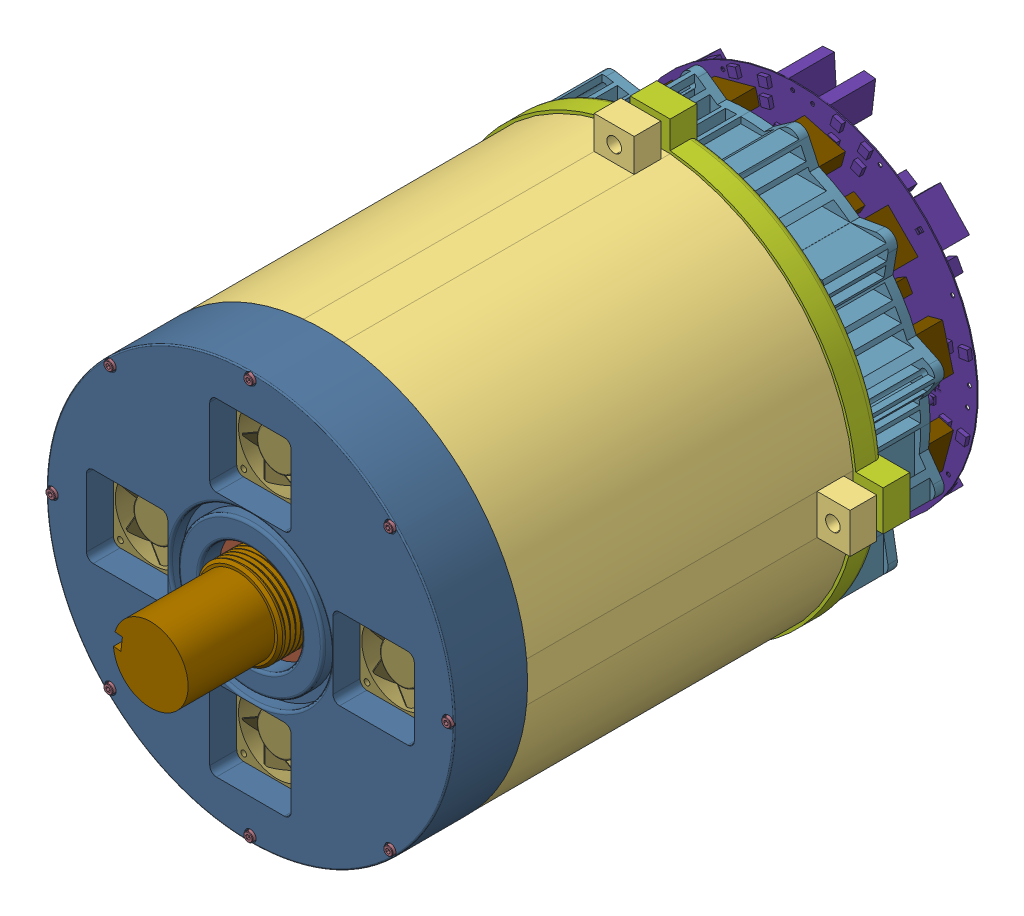
SolidWorks assembly motor assembly, configuration Varsayılan. Lengths in mm.
Overall size (354 354 520.07).
111 component instances, 18 part files, 52 mates.
Components (placement in the parent):
- stator-1: stator [Varsayılan] at (-45.285 13.1183 202.5) size (270 270 135)
- coil-1: coil [Varsayılan] at (-45.285 -93.8817 270) size (21.5 30 205)
- coil-2: coil [Varsayılan] at (-17.5914 -90.2358 270) x (0.965926 0.258819 0) z (0 0 1) size (21.5 30 205)
- coil-3: coil [Varsayılan] at (8.215 -79.5464 270) x (0.866025 0.5 0) z (0 0 1) size (21.5 30 205)
- coil-4: coil [Varsayılan] at (30.3754 -62.5422 270) x (0.707107 0.707107 0) z (0 0 1) size (21.5 30 205)
- coil-5: coil [Varsayılan] at (47.3797 -40.3817 270) x (0.5 0.866025 0) z (0 0 1) size (21.5 30 205)
- coil-6: coil [Varsayılan] at (58.0691 -14.5754 270) x (0.258819 0.965926 0) z (0 0 1) size (21.5 30 205)
- coil-7: coil [Varsayılan] at (61.715 13.1183 270) x (0 1 0) z (0 0 1) size (21.5 30 205)
- coil-8: coil [Varsayılan] at (58.0691 40.8119 270) x (-0.258819 0.965926 0) z (0 0 1) size (21.5 30 205)
- coil-9: coil [Varsayılan] at (47.3797 66.6183 270) x (-0.5 0.866025 0) z (0 0 1) size (21.5 30 205)
- coil-10: coil [Varsayılan] at (30.3754 88.7787 270) x (-0.707107 0.707107 0) z (0 0 1) size (21.5 30 205)
- coil-11: coil [Varsayılan] at (8.215 105.783 270) x (-0.866025 0.5 0) z (0 0 1) size (21.5 30 205)
- coil-12: coil [Varsayılan] at (-17.5914 116.4723 270) x (-0.965926 0.258819 0) z (0 0 1) size (21.5 30 205)
- coil-13: coil [Varsayılan] at (-45.285 120.1183 270) x (-1 0 0) z (0 0 1) size (21.5 30 205)
- coil-14: coil [Varsayılan] at (-72.9786 116.4723 270) x (-0.965926 -0.258819 0) z (0 0 1) size (21.5 30 205)
- coil-15: coil [Varsayılan] at (-98.785 105.783 270) x (-0.866025 -0.5 0) z (0 0 1) size (21.5 30 205)
- coil-16: coil [Varsayılan] at (-120.9454 88.7787 270) x (-0.707107 -0.707107 0) z (0 0 1) size (21.5 30 205)
- coil-17: coil [Varsayılan] at (-137.9497 66.6183 270) x (-0.5 -0.866025 0) z (0 0 1) size (21.5 30 205)
- coil-18: coil [Varsayılan] at (-148.6391 40.8119 270) x (-0.258819 -0.965926 0) z (0 0 1) size (21.5 30 205)
- coil-19: coil [Varsayılan] at (-152.285 13.1183 270) x (0 -1 0) z (0 0 1) size (21.5 30 205)
- coil-20: coil [Varsayılan] at (-148.6391 -14.5754 270) x (0.258819 -0.965926 0) z (0 0 1) size (21.5 30 205)
- coil-21: coil [Varsayılan] at (-137.9497 -40.3817 270) x (0.5 -0.866025 0) z (0 0 1) size (21.5 30 205)
- coil-22: coil [Varsayılan] at (-120.9454 -62.5422 270) x (0.707107 -0.707107 0) z (0 0 1) size (21.5 30 205)
- coil-23: coil [Varsayılan] at (-98.785 -79.5464 270) x (0.866025 -0.5 0) z (0 0 1) size (21.5 30 205)
- coil-24: coil [Varsayılan] at (-72.9786 -90.2358 270) x (0.965926 -0.258819 0) z (0 0 1) size (21.5 30 205)
- case-1: case [Varsayılan] at (-45.285 13.1183 390) x (-1 0 0) z (0 -1 0) size (354 245 354)
- rotor assembly-1: rotor assembly [Varsayılan] at (-60.6102 4.0993 71.3059) x (0.997912 -0.064595 0) z (0 0 1) size (229.36 229.36 135)
  - rotor core 1-1: rotor core 1 [Varsayılan] at (14.7106 9.9901 131.1941) size (164.94 164.94 67.5)
  - rotor core 2-1: rotor core 2 [Varsayılan] at (14.7106 9.9901 266.1941) x (0.824126 0.566406 0) z (0 0 -1) size (164.94 164.94 67.5)
  - magnet_67.5-1: magnet_67.5 [Varsayılan] at (14.7106 9.9901 198.6941) x (0.999657 -0.026177 0) z (0 0 1) size (19.71 16.61 67.5)
  - magnet_67.5-2: magnet_67.5 [Varsayılan] at (14.7106 9.9901 198.6941) x (0.95882 0.284015 0) z (0 0 1) size (19.71 16.61 67.5)
  - magnet_67.5-3: magnet_67.5 [Varsayılan] at (14.7106 9.9901 198.6941) x (0.824126 0.566406 0) z (0 0 1) size (19.71 16.61 67.5)
  - magnet_67.5-4: magnet_67.5 [Varsayılan] at (14.7106 9.9901 198.6941) x (0.608761 0.793353 0) z (0 0 1) size (19.71 16.61 67.5)
  - magnet_67.5-5: magnet_67.5 [Varsayılan] at (14.7106 9.9901 198.6941) x (0.333807 0.942641 0) z (0 0 1) size (19.71 16.61 67.5)
  - magnet_67.5-6: magnet_67.5 [Varsayılan] at (14.7106 9.9901 198.6941) x (0.026177 0.999657 0) z (0 0 1) size (19.71 16.61 67.5)
  - magnet_67.5-7: magnet_67.5 [Varsayılan] at (14.7106 9.9901 198.6941) x (-0.284015 0.95882 0) z (0 0 1) size (19.71 16.61 67.5)
  - magnet_67.5-8: magnet_67.5 [Varsayılan] at (14.7106 9.9901 198.6941) x (-0.566406 0.824126 0) z (0 0 1) size (19.71 16.61 67.5)
  - magnet_67.5-9: magnet_67.5 [Varsayılan] at (14.7106 9.9901 198.6941) x (-0.793353 0.608761 0) z (0 0 1) size (19.71 16.61 67.5)
  - magnet_67.5-10: magnet_67.5 [Varsayılan] at (14.7106 9.9901 198.6941) x (-0.942641 0.333807 0) z (0 0 1) size (19.71 16.61 67.5)
  - magnet_67.5-11: magnet_67.5 [Varsayılan] at (14.7106 9.9901 198.6941) x (-0.999657 0.026177 0) z (0 0 1) size (19.71 16.61 67.5)
  - magnet_67.5-12: magnet_67.5 [Varsayılan] at (14.7106 9.9901 198.6941) x (-0.95882 -0.284015 0) z (0 0 1) size (19.71 16.61 67.5)
  - magnet_67.5-13: magnet_67.5 [Varsayılan] at (14.7106 9.9901 198.6941) x (-0.824126 -0.566406 0) z (0 0 1) size (19.71 16.61 67.5)
  - magnet_67.5-14: magnet_67.5 [Varsayılan] at (14.7106 9.9901 198.6941) x (-0.608761 -0.793353 0) z (0 0 1) size (19.71 16.61 67.5)
  - magnet_67.5-15: magnet_67.5 [Varsayılan] at (14.7106 9.9901 198.6941) x (-0.333807 -0.942641 0) z (0 0 1) size (19.71 16.61 67.5)
  - magnet_67.5-16: magnet_67.5 [Varsayılan] at (14.7106 9.9901 198.6941) x (-0.026177 -0.999657 0) z (0 0 1) size (19.71 16.61 67.5)
  - magnet_67.5-17: magnet_67.5 [Varsayılan] at (14.7106 9.9901 198.6941) x (0.284015 -0.95882 0) z (0 0 1) size (19.71 16.61 67.5)
  - magnet_67.5-18: magnet_67.5 [Varsayılan] at (14.7106 9.9901 198.6941) x (0.566406 -0.824126 0) z (0 0 1) size (19.71 16.61 67.5)
  - magnet_67.5-19: magnet_67.5 [Varsayılan] at (14.7106 9.9901 198.6941) x (0.793353 -0.608761 0) z (0 0 1) size (19.71 16.61 67.5)
  - magnet_67.5-20: magnet_67.5 [Varsayılan] at (14.7106 9.9901 198.6941) x (0.942641 -0.333807 0) z (0 0 1) size (19.71 16.61 67.5)
  - magnet_67.5-21: magnet_67.5 [Varsayılan] at (14.7106 9.9901 131.1941) size (19.71 16.61 67.5)
  - magnet_67.5-22: magnet_67.5 [Varsayılan] at (14.7106 9.9901 131.1941) x (0.951057 -0.309017 0) z (0 0 1) size (19.71 16.61 67.5)
  - magnet_67.5-23: magnet_67.5 [Varsayılan] at (14.7106 9.9901 131.1941) x (0.809017 -0.587785 0) z (0 0 1) size (19.71 16.61 67.5)
  - magnet_67.5-24: magnet_67.5 [Varsayılan] at (14.7106 9.9901 131.1941) x (0.587785 -0.809017 0) z (0 0 1) size (19.71 16.61 67.5)
  - magnet_67.5-25: magnet_67.5 [Varsayılan] at (14.7106 9.9901 131.1941) x (0.309017 -0.951057 0) z (0 0 1) size (19.71 16.61 67.5)
  - magnet_67.5-26: magnet_67.5 [Varsayılan] at (14.7106 9.9901 131.1941) x (0 -1 0) z (0 0 1) size (19.71 16.61 67.5)
  - magnet_67.5-27: magnet_67.5 [Varsayılan] at (14.7106 9.9901 131.1941) x (-0.309017 -0.951057 0) z (0 0 1) size (19.71 16.61 67.5)
  - magnet_67.5-28: magnet_67.5 [Varsayılan] at (14.7106 9.9901 131.1941) x (-0.587785 -0.809017 0) z (0 0 1) size (19.71 16.61 67.5)
  - magnet_67.5-29: magnet_67.5 [Varsayılan] at (14.7106 9.9901 131.1941) x (-0.809017 -0.587785 0) z (0 0 1) size (19.71 16.61 67.5)
  - magnet_67.5-30: magnet_67.5 [Varsayılan] at (14.7106 9.9901 131.1941) x (-0.951057 -0.309017 0) z (0 0 1) size (19.71 16.61 67.5)
  - magnet_67.5-31: magnet_67.5 [Varsayılan] at (14.7106 9.9901 131.1941) x (-1 0 0) z (0 0 1) size (19.71 16.61 67.5)
  - magnet_67.5-32: magnet_67.5 [Varsayılan] at (14.7106 9.9901 131.1941) x (-0.951057 0.309017 0) z (0 0 1) size (19.71 16.61 67.5)
  - magnet_67.5-33: magnet_67.5 [Varsayılan] at (14.7106 9.9901 131.1941) x (-0.809017 0.587785 0) z (0 0 1) size (19.71 16.61 67.5)
  - magnet_67.5-34: magnet_67.5 [Varsayılan] at (14.7106 9.9901 131.1941) x (-0.587785 0.809017 0) z (0 0 1) size (19.71 16.61 67.5)
  - magnet_67.5-35: magnet_67.5 [Varsayılan] at (14.7106 9.9901 131.1941) x (-0.309017 0.951057 0) z (0 0 1) size (19.71 16.61 67.5)
  - magnet_67.5-36: magnet_67.5 [Varsayılan] at (14.7106 9.9901 131.1941) x (0 1 0) z (0 0 1) size (19.71 16.61 67.5)
  - magnet_67.5-37: magnet_67.5 [Varsayılan] at (14.7106 9.9901 131.1941) x (0.309017 0.951057 0) z (0 0 1) size (19.71 16.61 67.5)
  - magnet_67.5-38: magnet_67.5 [Varsayılan] at (14.7106 9.9901 131.1941) x (0.587785 0.809017 0) z (0 0 1) size (19.71 16.61 67.5)
  - magnet_67.5-39: magnet_67.5 [Varsayılan] at (14.7106 9.9901 131.1941) x (0.809017 0.587785 0) z (0 0 1) size (19.71 16.61 67.5)
  - magnet_67.5-40: magnet_67.5 [Varsayılan] at (14.7106 9.9901 131.1941) x (0.951057 0.309017 0) z (0 0 1) size (19.71 16.61 67.5)
- arka kapak zgr-1: arka kapak zgr [Default] at (-45.285 13.1183 160) x (0 0 -1) z (1 0 0) size (35.23 349.6 349.6)
- 6205 rulman-1: 6205 rulman [Varsayılan] at (-45.285 13.1183 135) x (0.999542 -0.030267 0) z (0 0 1) size (62 62 16)
- mıl-1: mıl [Default] at (-45.285 13.1183 499.75) x (0 0 1) z (-0.111143 -0.993804 0) size (443 80 80)
- on kapak-1: on kapak [Default] at (-45.285 13.1183 380) size (306 306 65)
- 6212 rulman-1: 6212 rulman [Default] at (-45.285 13.1183 408) size (110 110 22)
- 6212 rulman-2: 6212 rulman [Default] at (-45.285 13.1183 386) x (0.99317 -0.116678 0) z (0 0 1) size (110 110 22)
- Fan-60x60-1: Fan-60x60 [25mm] at (-45.285 105.6183 406.0237) size (71.21 64.96 25)
- Fan-60x60-2: Fan-60x60 [25mm] at (-137.785 13.1183 406.0237) x (0 1 0) z (0 0 1) size (71.21 64.96 25)
- Fan-60x60-3: Fan-60x60 [25mm] at (-45.285 -79.3817 406.0237) x (-1 0 0) z (0 0 1) size (71.21 64.96 25)
- Fan-60x60-4: Fan-60x60 [25mm] at (47.215 13.1183 406.0237) x (0 -1 0) z (0 0 1) size (71.21 64.96 25)
- Fan-60x60-5: Fan-60x60 [25mm] at (-101.8535 69.6868 131.0283) x (0 -1 0) z (0 0 1) size (71.21 64.96 25)
- socket head cap screw_am-1: socket head cap screw_am [B18.3.1M - 4 x 0.7 x 30 Hex SHCS -- 20CHX] at (63.0994 -49.154 42.8) x (0 0 1) z (0.759805 0.650151 0) size (34 7 7)
- socket head cap screw_am-3: socket head cap screw_am [B18.3.1M - 4 x 0.7 x 30 Hex SHCS -- 20CHX] at (75.3874 45.7245 42.8) x (0 0 1) z (0.077537 0.99699 0) size (34 7 7) (hidden)
- socket head cap screw_am-4: socket head cap screw_am [B18.3.1M - 4 x 0.7 x 30 Hex SHCS -- 20CHX] at (16.9872 121.5026 42.8) x (0 0 1) z (-0.650151 0.759805 0) size (34 7 7) (hidden)
- socket head cap screw_am-5: socket head cap screw_am [B18.3.1M - 4 x 0.7 x 30 Hex SHCS -- 20CHX] at (-77.8912 133.7907 42.8) x (0 0 1) z (-0.99699 0.077537 0) size (34 7 7) (hidden)
- socket head cap screw_am-6: socket head cap screw_am [B18.3.1M - 4 x 0.7 x 30 Hex SHCS -- 20CHX] at (-153.6694 75.3905 42.8) x (0 0 1) z (-0.759805 -0.650151 0) size (34 7 7) (hidden)
- socket head cap screw_am-7: socket head cap screw_am [B18.3.1M - 4 x 0.7 x 30 Hex SHCS -- 20CHX] at (-165.9574 -19.4879 42.8) x (0 0 1) z (-0.077537 -0.99699 0) size (34 7 7) (hidden)
- socket head cap screw_am-8: socket head cap screw_am [B18.3.1M - 4 x 0.7 x 30 Hex SHCS -- 20CHX] at (-107.5572 -95.2661 42.8) x (0 0 1) z (0.650151 -0.759805 0) size (34 7 7) (hidden)
- socket head cap screw_am-9: socket head cap screw_am [B18.3.1M - 4 x 0.7 x 30 Hex SHCS -- 20CHX] at (-12.6788 -107.5542 42.8) x (0 0 1) z (0.99699 -0.077537 0) size (34 7 7) (hidden)
- Fan-60x60-12: Fan-60x60 [25mm] at (-101.8535 -43.4503 131.0283) size (71.21 64.96 25)
- Fan-60x60-13: Fan-60x60 [25mm] at (11.2835 -43.4503 131.0283) x (0 1 0) z (0 0 1) size (71.21 64.96 25)
- Fan-60x60-14: Fan-60x60 [25mm] at (11.2835 69.6868 131.0283) x (-1 0 0) z (0 0 1) size (71.21 64.96 25)
- HeatSinkOneModule_mst-2: HeatSinkOneModule_mst [Varsayılan] at (-45.285 13.1183 70) x (1 0 0) z (0 -1 0) size (145.64 55 145.64)
- HeatSinkOneModule_mst-3: HeatSinkOneModule_mst [Varsayılan] at (-45.285 13.1183 70) x (0 1 0) z (1 0 0) size (145.64 55 145.64)
- HeatSinkOneModule_mst-4: HeatSinkOneModule_mst [Varsayılan] at (-45.285 13.1183 70) x (-1 0 0) z (0 1 0) size (145.64 55 145.64)
- HeatSinkOneModule_mst-5: HeatSinkOneModule_mst [Varsayılan] at (-45.285 13.1183 70) x (0 -1 0) z (-1 0 0) size (145.64 55 145.64)
- encoder_assem-1: encoder_assem [Varsayılan] at (-49.9209 11.8321 164) x (-0.034519 0.999404 0) z (0 0 -1) size (52.69 74.69 46.7)
  - encoder_body-1: encoder_body [Varsayılan] at (1.1254 4.6776 50) size (50 50 44.7)
  - encoder_bracket-1: encoder_bracket [Varsayılan] at (1.1254 4.6776 49.9) x (0 0 -1) z (-0.999404 -0.034519 0) size (11 73 50.2)
- ControlBoard-1: ControlBoard [Varsayılan] at (-45.2858 13.1179 33.7804) x (-0.027373 -0.999625 0) z (0 0 -1) size (270 270 45.4)
- GD_Layout-1: GD_Layout [Varsayılan] at (-45.2843 13.119 68.5789) x (0 1 0) z (0 0 -1) size (133 133 24.37)
- GD_Layout-2: GD_Layout [Varsayılan] at (-45.285 13.1183 68.5789) x (1 0 0) z (0 0 -1) size (133 133 24.37)
- GD_Layout-3: GD_Layout [Varsayılan] at (-45.285 13.1183 68.5789) x (0 -1 0) z (0 0 -1) size (133 133 24.37)
- GD_Layout-4: GD_Layout [Varsayılan] at (-45.2857 13.119 68.5789) x (-1 0 0) z (0 0 -1) size (133 133 24.37)
- socket head cap screw_am-10: socket head cap screw_am [B18.3.1M - 4 x 0.7 x 80 Hex SHCS -- 20NHX] at (-45.285 161.5955 446.8) x (0 0 -1) z (0.019286 0.999814 0) size (84 7 7)
- socket head cap screw_am-11: socket head cap screw_am [B18.3.1M - 4 x 0.7 x 80 Hex SHCS -- 20NHX] at (-150.2742 118.1075 446.8) x (0 0 -1) z (-0.693338 0.720612 0) size (84 7 7)
- socket head cap screw_am-12: socket head cap screw_am [B18.3.1M - 4 x 0.7 x 80 Hex SHCS -- 20NHX] at (-193.7622 13.1183 446.8) x (0 0 -1) z (-0.999814 0.019286 0) size (84 7 7)
- socket head cap screw_am-13: socket head cap screw_am [B18.3.1M - 4 x 0.7 x 80 Hex SHCS -- 20NHX] at (-150.2742 -91.8709 446.8) x (0 0 -1) z (-0.720612 -0.693338 0) size (84 7 7)
- socket head cap screw_am-14: socket head cap screw_am [B18.3.1M - 4 x 0.7 x 80 Hex SHCS -- 20NHX] at (-45.285 -135.3589 446.8) x (0 0 -1) z (-0.019286 -0.999814 0) size (84 7 7)
- socket head cap screw_am-15: socket head cap screw_am [B18.3.1M - 4 x 0.7 x 80 Hex SHCS -- 20NHX] at (59.7042 -91.8709 446.8) x (0 0 -1) z (0.693338 -0.720612 0) size (84 7 7)
- socket head cap screw_am-16: socket head cap screw_am [B18.3.1M - 4 x 0.7 x 80 Hex SHCS -- 20NHX] at (103.1922 13.1183 446.8) x (0 0 -1) z (0.999814 -0.019286 0) size (84 7 7)
- socket head cap screw_am-17: socket head cap screw_am [B18.3.1M - 4 x 0.7 x 80 Hex SHCS -- 20NHX] at (59.7042 118.1075 446.8) x (0 0 -1) z (0.720612 0.693338 0) size (84 7 7)
Mates (geometry in assembly coordinates):
- Width1: width: plane of coil-1 through (-38.535 -78.8817 270) normal (-1 0 0); plane of coil-1 through (-52.035 -78.8817 361.8) normal (1 0 0); plane of stator-1 through (-39.0069 -108.9108 337.5) normal (1 0 0); plane of stator-1 through (-51.5631 -76.6625 337.5) normal (-1 0 0)
- Width2: width: plane of stator-1 through (-45.285 13.1183 202.5) normal (0 0 -1); plane of stator-1 through (-45.285 13.1183 337.5) normal (0 0 1); plane of coil-1 through (-45.235 -78.8817 368.5) normal (0 0 -1); plane of coil-1 through (-45.335 -78.8817 171.5) normal (0 0 1)
- Distance1: distance = 2 mm: plane of coil-1 through (-52.035 -78.8817 361.8) normal (0 1 0); cylinder of stator-1 through (-45.285 13.1183 337.5) axis (0 0 -1) radius 90
- Concentric1: concentric: circle of stator-1; circle of case-1
- Concentric4: concentric: circle of case-1; circle of rotor assembly-1/rotor core 2-1
- Coincident4: coincident: plane of stator-1 through (-45.285 13.1183 337.5) normal (0 0 1); plane of rotor assembly-1/magnet_67.5-18 through (-45.285 13.1183 337.5) normal (0 0 1)
- Coincident6: coincident: plane of case-1 through (-45.285 13.1183 145) normal (0 0 -1); plane of arka kapak zgr-1 through (-45.285 168.1183 145) normal (0 0 1)
- Coincident7: coincident: plane of rotor assembly-1/rotor core 2-1 through (-45.285 13.1183 303.75) normal (0 0 1); plane of mıl-1 through (-85.0372 17.564 303.75) normal (0 0 -1)
- Concentric10: concentric: circle of on kapak-1; circle of 6212 rulman-1
- Coincident8: coincident: plane of on kapak-1 through (-45.285 13.1183 430) normal (0 0 -1); plane of 6212 rulman-1 through (-45.285 13.1183 430) normal (0 0 1)
- Concentric11: concentric: circle of on kapak-1; circle of 6212 rulman-2
- Coincident9: coincident: plane of 6212 rulman-1 through (-45.285 13.1183 408) normal (0 0 -1); plane of 6212 rulman-2 through (-45.285 13.1183 408) normal (0 0 1)
- Coincident10: coincident: plane of case-1 through (-45.285 13.1183 390) normal (0 0 1); plane of on kapak-1 through (-45.285 13.1183 390) normal (0 0 -1)
- Parallel1: parallel: line of arka kapak zgr-1 through (-19.2165 95.1868 125) axis (0 -1 0); line of on kapak-1 through (-14.785 131.1183 445) axis (0 -1 0)
- Distance2: distance = 10 mm: plane of arka kapak zgr-1 through (-45.285 13.1183 120) normal (0 0 -1); plane of ? through (620.715 -151.8817 110) normal (0 0 1)
- Parallel2: parallel: line of arka kapak zgr-1 through (-76.3535 -12.9503 120) axis (-1 0 0); line of ? through (-45.285 13.1183 55) axis (-1 0 0)
- Width5: width: plane of on kapak-1 through (-45.285 136.1183 445) normal (0 -1 0); plane of on kapak-1 through (-45.285 75.1183 445) normal (0 1 0); plane of Fan-60x60-1 through (-20.285 135.8723 424.9954) normal (0 1 0); plane of Fan-60x60-1 through (-20.285 75.3643 424.9954) normal (0 -1 0)
- Perpendicular1: perpendicular: plane of coil-13 through (-34.535 105.1183 361.8) normal (1 0 0); plane of on kapak-1 through (-45.285 80.1183 445) normal (0 1 0)
- Width6: width: plane of on kapak-1 through (-75.785 13.1183 445) normal (1 0 0); plane of on kapak-1 through (-14.785 13.1183 445) normal (-1 0 0); plane of Fan-60x60-1 through (-75.539 80.6183 424.9954) normal (-1 0 0); plane of Fan-60x60-1 through (-15.031 80.6183 424.9954) normal (1 0 0)
- Coincident14: coincident: plane of on kapak-1 through (-45.285 13.1183 400) normal (0 0 1); plane of Fan-60x60-1 through (-70.2872 130.6202 400) normal (0 0 -1)
- Width7: width: plane of Fan-60x60-5 through (-71.5995 44.6868 150) normal (1 0 0); plane of Fan-60x60-5 through (-132.1075 44.6868 150) normal (-1 0 0); plane of arka kapak zgr-1 through (-71.3535 95.1868 125) normal (-1 0 0); plane of arka kapak zgr-1 through (-132.3535 95.1868 125) normal (1 0 0)
- Width8: width: plane of Fan-60x60-5 through (-126.8535 99.9408 150) normal (0 1 0); plane of Fan-60x60-5 through (-126.8535 39.4328 150) normal (0 -1 0); plane of arka kapak zgr-1 through (-127.3535 100.1868 125) normal (0 -1 0); plane of arka kapak zgr-1 through (-127.3535 39.1868 125) normal (0 1 0)
- Coincident16: coincident: plane of arka kapak zgr-1 through (-127.3535 44.1868 150) normal (0 0 -1); plane of Fan-60x60-5 through (-126.8564 44.6842 150) normal (0 0 1)
- Distance3: distance = 20 mm: plane of ? through (-45.285 13.1183 68.4) normal (0 0 -1); plane of ? through (-45.285 13.1183 48.4) normal (0 0 1)
- Concentric16: concentric: circle of ?; circle of socket head cap screw_am-1
- Coincident24: coincident: plane of ? through (-45.285 13.1183 46.8) normal (0 0 -1); plane of socket head cap screw_am-1 through (52.4148 -70.2826 46.8) normal (0 0 1)
- Concentric22: concentric: circle of rotor assembly-1/rotor core 2-1; circle of mıl-1
- Concentric23: concentric: circle of mıl-1; circle of on kapak-1
- Parallel5: parallel: line of coil-7 through (76.715 13.0683 167.5) axis (-1 0 0); line of case-1 through (-60.285 190.1183 152) axis (1 0 0)
- Concentric24: concentric: circle of arka kapak zgr-1; circle of mıl-1
- Concentric25: concentric: circle of arka kapak zgr-1; circle of ?
- Distance4: distance = 0 mm: plane of arka kapak zgr-1 through (-45.285 13.1183 120) normal (0 0 -1); plane of ? through (-29.9967 -986.7649 120) normal (0 0 1)
- Coincident26: coincident: plane of arka kapak zgr-1 through (-45.285 29.1183 125) normal (0 0 -1); plane of HeatSinkOneModule_mst-2 through (-45.285 -986.8817 125) normal (0 0 1)
- Parallel6: parallel: plane of arka kapak zgr-1 through (-60.285 13.1183 145) normal (-1 0 0); plane of HeatSinkOneModule_mst-2 through (-45.285 -986.8817 70) normal (-1 0 0)
- Coincident27: coincident: plane of ? through (-45.285 13.1183 70) normal (0 0 1); plane of HeatSinkOneModule_mst-2 through (-45.285 -986.8817 70) normal (0 0 -1)
- Concentric28: concentric: circle of ?; circle of ?
- Concentric29: concentric: circle of mıl-1; circle of encoder_assem-1/encoder_body-1
- Coincident28: coincident: plane of arka kapak zgr-1 through (-45.285 29.1183 125) normal (0 0 -1); plane of encoder_assem-1/encoder_bracket-1 through (-70.185 13.1183 125) normal (0 0 1)
- Parallel8: parallel: line of arka kapak zgr-1 through (-220.085 28.1183 125) axis (1 0 0); line of encoder_assem-1/encoder_bracket-1 through (-68.3069 23.1183 124.8) axis (-1 0 0)
- Concentric31: concentric: circle of mıl-1; circle of HeatSinkOneModule_mst-3
- Concentric32: concentric: circle of ?; circle of HeatSinkOneModule_mst-2
- Parallel9: parallel: plane of ? through (-45.285 13.1183 68.4) normal (-1 0 0); plane of HeatSinkOneModule_mst-2 through (-45.285 -986.8817 70) normal (-1 0 0)
- Concentric33: concentric: circle of rotor assembly-1/rotor core 1-1; circle of 6205 rulman-1
- Distance6: distance = 16 mm: plane of arka kapak zgr-1 through (-45.285 44.1183 135) normal (0 0 1); plane of 6205 rulman-1 through (-45.285 13.1183 151) normal (0 0 1)
- Width9: width: plane of on kapak-1 through (-45.285 13.1183 380) normal (0 0 -1); plane of arka kapak zgr-1 through (-45.285 146.1183 160) normal (0 0 1); plane of stator-1 through (-45.285 13.1183 202.5) normal (0 0 -1); plane of stator-1 through (-45.285 13.1183 337.5) normal (0 0 1)
- Concentric34: concentric: circle of HeatSinkOneModule_mst-3; circle of GD_Layout-1
- Çakışık1: coincident: plane of HeatSinkOneModule_mst-3 through (954.715 13.1183 70) normal (0 0 -1); plane of GD_Layout-1 through (-7.943 103.6119 70) normal (0 0 1)
- Çakışık2: coincident: line of HeatSinkOneModule_mst-3 through (89.715 13.1183 70) axis (-1 0 0); plane of GD_Layout-1 through (-35.2843 13.119 69.5703) normal (0 -1 0)
- Eş Merkezli1: concentric: circle of ControlBoard-1; circle of GD_Layout-3
- Uzaklık1: distance = 10 mm: plane of ControlBoard-1 through (2.7154 129.7709 37.5789) normal (0 0 1); plane of GD_Layout-2 through (65.8205 -33.0194 47.5789) normal (0 0 -1)
- Eş Merkezli13: concentric: circle of on kapak-1; circle of socket head cap screw_am-10
- Çakışık16: coincident: plane of on kapak-1 through (-43.035 161.5955 442.8) normal (0 0 1); plane of socket head cap screw_am-10 through (-48.7843 161.663 442.8) normal (0 0 -1)
